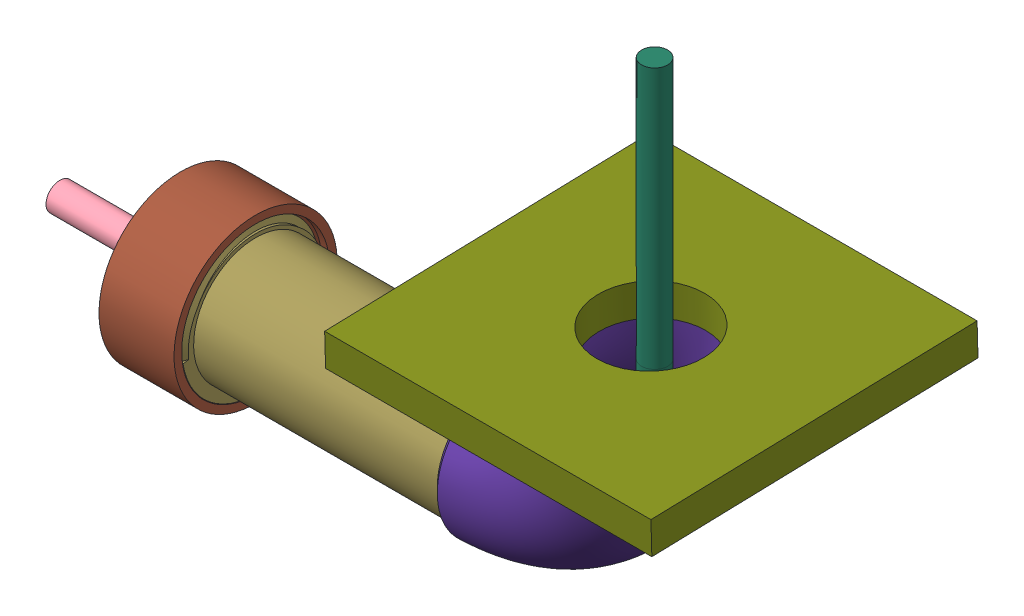
SolidWorks assembly new feedthrough 4, configuration Default. Lengths in mm.
Overall size (232.75 164.52 100.24).
30 component instances, 17 part files, 31 mates.
Components (placement in the parent):
- PCB-1: PCB [Default] at origin size (2 20 20)
- 1424177.stp-1: 1424177.stp [Default] at (6.35 0 0) x (0 -0.707107 0.707107) z (-1 0 0) size (27.6 26.9 24.95)
  - BS-BF-HW-BUCHSE-CAT6A_SW0001.stp-1: BS-BF-HW-BUCHSE-CAT6A_SW0001.stp [Default] at origin size (17.2 20.01 24.95)
  - 415371.stp-1: 415371.stp [Default] at (0 0 -8.45) x (-0.866025 -0.5 0) z (0 0 -1) size (20.9 19 2.8)
- cable assem-1: cable assem [Default] at (-53.2936 -50.2297 -9.5758) x (1 0 0) z (0 0.707107 0.707107) size (73.59 15.36 15.36)
  - cable-1: cable [Default] at (41.7936 28.7467 42.2889) x (0 0 1) z (-1 0 0) size (8.5 8.5 60.1)
  - 2 wires-1: 2 wires [Default] at (41.7936 28.7467 42.2889) x (0 1 0) z (1 0 0) size (5.09 5.18 13.49)
  - 2 wires-2: 2 wires [Default] at (41.7936 28.7467 42.2889) x (0 0 1) z (1 0 0) size (5.09 5.18 13.49)
  - 2 wires-3: 2 wires [Default] at (41.7936 28.7467 42.2889) x (0 -1 0) z (1 0 0) size (5.09 5.18 13.49)
  - 2 wires-4: 2 wires [Default] at (41.7936 28.7467 42.2889) x (0 0 -1) z (1 0 0) size (5.09 5.18 13.49)
- outer flange-2: outer flange [Default] at (-29 0 0) x (-1 0 0) z (0 0.711666 -0.702518) size (28 41.9 41.9)
- end cap-1: end cap [Default] at (-17.5 0 0) x (1 0 0) z (0 0.006202 0.999981) size (4 12 12)
- end cap-2: end cap [Default] at (-43.5 0 0) x (-1 0 0) z (0 -0.926575 -0.37611) size (4 12 12)
- support plate-1: support plate [Default] at (11 0 0) x (0 0.006469 -0.999979) z (0 0.999979 0.006469) size (31 4 31)
- 92290A058_Super-Corrosion-Resistant 316 Stainless Steel Socket Head Screw-1: 92290A058_Super-Corrosion-Resistant 316 Stainless Steel Socket Head Screw [92290A058] at (3 0.0841 -12.9997) x (0 0.578122 0.81595) z (-1 0 0) size (4.5 4.5 10.62)
- 93655A361_Male-Female Threaded Hex Standoff-1: 93655A361_Male-Female Threaded Hex Standoff [93655A361] at (-10.45 0.0841 -12.9997) x (-1 0 0) z (0 0.711178 -0.703012) size (34.9 5.2 4.5)
- 92290A058_Super-Corrosion-Resistant 316 Stainless Steel Socket Head Screw-8: 92290A058_Super-Corrosion-Resistant 316 Stainless Steel Socket Head Screw [92290A058] at (3 12.9997 0.0841) x (0 -0.81595 0.578122) z (-1 0 0) size (4.5 4.5 10.62)
- 92290A058_Super-Corrosion-Resistant 316 Stainless Steel Socket Head Screw-9: 92290A058_Super-Corrosion-Resistant 316 Stainless Steel Socket Head Screw [92290A058] at (3 -0.0841 12.9997) x (0 -0.578122 -0.81595) z (-1 0 0) size (4.5 4.5 10.62)
- 92290A058_Super-Corrosion-Resistant 316 Stainless Steel Socket Head Screw-10: 92290A058_Super-Corrosion-Resistant 316 Stainless Steel Socket Head Screw [92290A058] at (3 -12.9997 -0.0841) x (0 0.81595 -0.578122) z (-1 0 0) size (4.5 4.5 10.62)
- 93655A361_Male-Female Threaded Hex Standoff-8: 93655A361_Male-Female Threaded Hex Standoff [93655A361] at (-10.45 12.9997 0.0841) x (-1 0 0) z (0 0.703012 0.711178) size (34.9 5.2 4.5)
- 93655A361_Male-Female Threaded Hex Standoff-9: 93655A361_Male-Female Threaded Hex Standoff [93655A361] at (-10.45 -0.0841 12.9997) x (-1 0 0) z (0 -0.711178 0.703012) size (34.9 5.2 4.5)
- 93655A361_Male-Female Threaded Hex Standoff-10: 93655A361_Male-Female Threaded Hex Standoff [93655A361] at (-10.45 -12.9997 -0.0841) x (-1 0 0) z (0 -0.703012 -0.711178) size (34.9 5.2 4.5)
- flange cover-1: flange cover [Default] at (-34.5 0 0) x (0 0.640688 -0.767801) z (0 -0.767801 -0.640688) size (50 23 50)
- innder flange-1: innder flange [Default] at (-26.5 0 0) x (0 0.988801 0.149242) z (0 0.149242 -0.988801) size (46.1 91.5 45.01)
- M12 cable-1: M12 cable [Default] at (12.9 0 0) x (-1 0 0) z (0 -0.986189 0.165625) size (101.9 33.14 134.89)
  - M12 cable a-1: M12 cable a [Default] at origin size (29.9 16 16)
  - M12 cable b-1: M12 cable b [Default] at (5 0 0) size (20 15 15)
  - 8mm cable v4-1: 8mm cable v4 [Default] at (-44.9 0 0) x (1 0 0) z (0 0.986189 -0.165625) size (57 132 8)
- plate-1: plate [Default] at (111.252 47.7334 1.3309) x (1 0 0) z (0 -0.027872 0.999612) size (100 10 100)
- 45555K514_Standard-Wall Butt-Weld Unthreaded Pipe Fitting-1: 45555K514_Standard-Wall Butt-Weld Unthreaded Pipe Fitting [45555K514] at (63.5 47.7334 1.3309) x (0 0.999612 0.027872) z (0 0.027872 -0.999612) size (69.01 69.01 42.36)
Mates (geometry in assembly coordinates):
- Concentric1: concentric aligned: cylinder of PCB-1 through (2 3.5355 3.5355) axis (-1 0 0) radius 0.5; cylinder of 1424177.stp-1/BS-BF-HW-BUCHSE-CAT6A_SW0001.stp-1 through (2 3.5355 3.5355) axis (-1 0 0) radius 0.5
- Concentric2: concentric aligned: cylinder of PCB-1 through (2 -3.5355 3.5355) axis (-1 0 0) radius 0.5; cylinder of 1424177.stp-1/BS-BF-HW-BUCHSE-CAT6A_SW0001.stp-1 through (2 -3.5355 3.5355) axis (-1 0 0) radius 0.5
- Coincident1: coincident anti-aligned: plane of 1424177.stp-1/BS-BF-HW-BUCHSE-CAT6A_SW0001.stp-1 through (2 0 0) normal (-1 0 0); plane of PCB-1 through (2 0 0) normal (1 0 0)
- Concentric3: concentric aligned: cylinder of cable assem-1/cable-1 through (-71.5 0 0) axis (1 0 0) radius 4.25; cylinder of outer flange-2 through (-29 0 0) axis (1 0 0) radius 4.25
- Distance1: distance = 5 mm aligned: plane of cable assem-1/cable-1 through (-11.5 0 0) normal (1 0 0); plane of outer flange-2 through (-16.5 0 0) normal (1 0 0)
- Concentric4: concentric anti-aligned: cylinder of outer flange-2 through (-29 0 0) axis (1 0 0) radius 6; cylinder of end cap-1 through (-15.5023 0 0) axis (-1 0 0) radius 5
- Coincident3: coincident aligned: plane of outer flange-2 through (-16.5 0 0) normal (1 0 0); plane of end cap-1 through (-16.5 0 0) normal (1 0 0)
- Concentric5: concentric aligned: cylinder of outer flange-2 through (-29 0 0) axis (1 0 0) radius 6; cylinder of end cap-2 through (-45.4977 0 0) axis (1 0 0) radius 5
- Coincident4: coincident aligned: plane of outer flange-2 through (-44.5 0 0) normal (-1 0 0); plane of end cap-2 through (-44.5 0 0) normal (-1 0 0)
- Concentric21: concentric anti-aligned: cylinder of PCB-1 through (2 0 0) axis (-1 0 0) radius 10; cylinder of support plate-1 through (7 0 0) axis (1 0 0) radius 7
- Coincident10: coincident anti-aligned: plane of 1424177.stp-1/BS-BF-HW-BUCHSE-CAT6A_SW0001.stp-1 through (7 0 0) normal (1 0 0); plane of support plate-1 through (7 0 0) normal (-1 0 0)
- Concentric22: concentric anti-aligned: cylinder of support plate-1 through (7 0.0841 -12.9997) axis (1 0 0) radius 1.5; cylinder of 92290A058_Super-Corrosion-Resistant 316 Stainless Steel Socket Head Screw-1 through (11 0.0841 -12.9997) axis (-1 0 0) radius 1.25
- Coincident11: coincident anti-aligned: plane of support plate-1 through (11 0 0) normal (1 0 0); circle of 92290A058_Super-Corrosion-Resistant 316 Stainless Steel Socket Head Screw-1
- Coincident18: coincident anti-aligned: plane of outer flange-2 through (-24 0 0) normal (1 0 0); plane of 93655A361_Male-Female Threaded Hex Standoff-1 through (-24 1.9106 -11.152) normal (-1 0 0)
- Concentric27: concentric aligned: cylinder of outer flange-2 through (-29 0 0) axis (1 0 0) radius 7; circle of flange cover-1
- Coincident20: coincident anti-aligned: plane of outer flange-2 through (-31.5 0 0) normal (-1 0 0); plane of flange cover-1 through (-31.5 0 0) normal (1 0 0)
- Concentric28: concentric aligned: cylinder of flange cover-1 through (-11.5 0 0) axis (-1 0 0) radius 25; cylinder of innder flange-1 through (15.5 0 0) axis (-1 0 0) radius 16.5
- Coincident22: coincident aligned: plane of flange cover-1 through (-11.5 0 0) normal (1 0 0); plane of innder flange-1 through (-11.5 0 0) normal (1 0 0)
- Concentric30: concentric anti-aligned: cylinder of outer flange-2 through (-29 -0.0841 12.9997) axis (1 0 0) radius 1.25; cylinder of 93655A361_Male-Female Threaded Hex Standoff-9 through (-24 -0.0841 12.9997) axis (-1 0 0) radius 1.25
- Concentric31: concentric anti-aligned: cylinder of outer flange-2 through (-29 -12.9997 -0.0841) axis (1 0 0) radius 1.25; cylinder of 93655A361_Male-Female Threaded Hex Standoff-10 through (-24 -12.9997 -0.0841) axis (-1 0 0) radius 1.25
- Concentric32: concentric aligned: circle of 1424177.stp-1/BS-BF-HW-BUCHSE-CAT6A_SW0001.stp-1; circle of M12 cable-1/M12 cable a-1
- Coincident24: coincident anti-aligned: plane of 1424177.stp-1/BS-BF-HW-BUCHSE-CAT6A_SW0001.stp-1 through (23 0 0) normal (1 0 0); plane of M12 cable-1/M12 cable a-1 through (23 -1.0434 -6.213) normal (-1 0 0)
- Coincident25: coincident: line of M12 cable-1/8mm cable-1 through (110.8 48 0) axis (0 1 0)
- Parallel1: parallel anti-aligned: plane of plate-1 through (61.252 57.7296 1.6096) normal (-1 0 0)
- Concentric34: concentric anti-aligned: cylinder of 92290A058_Super-Corrosion-Resistant 316 Stainless Steel Socket Head Screw-8 through (11 12.9997 0.0841) axis (-1 0 0) radius 1.25; cylinder of 93655A361_Male-Female Threaded Hex Standoff-8 through (2.2 12.9997 0.0841) axis (1 0 0) radius 1.25
- Concentric35: concentric anti-aligned: cylinder of 92290A058_Super-Corrosion-Resistant 316 Stainless Steel Socket Head Screw-1 through (11 0.0841 -12.9997) axis (-1 0 0) radius 1.25; cylinder of 93655A361_Male-Female Threaded Hex Standoff-1 through (2.2 0.0841 -12.9997) axis (1 0 0) radius 1.25
- Coincident31: coincident anti-aligned: plane of support plate-1 through (7 0 0) normal (-1 0 0); plane of 93655A361_Male-Female Threaded Hex Standoff-1 through (7 1.9106 -11.152) normal (1 0 0)
- Concentric36: concentric aligned: circle of plate-1; circle of 45555K514_Standard-Wall Butt-Weld Unthreaded Pipe Fitting-1
- Coincident32: coincident anti-aligned: plane of plate-1 through (111.252 47.7334 1.3309) normal (0 -0.999612 -0.027872); plane of 45555K514_Standard-Wall Butt-Weld Unthreaded Pipe Fitting-1 through (111.252 47.7334 1.3309) normal (0 0.999612 0.027872)
- Concentric39: concentric aligned: cylinder of support plate-1 through (7 0 0) axis (1 0 0) radius 15.5; circle of 45555K514_Standard-Wall Butt-Weld Unthreaded Pipe Fitting-1
- Coincident34: coincident anti-aligned: plane of innder flange-1 through (63.5 0 0) normal (1 0 0); plane of 45555K514_Standard-Wall Butt-Weld Unthreaded Pipe Fitting-1 through (63.5 0 0) normal (-1 0 0)
